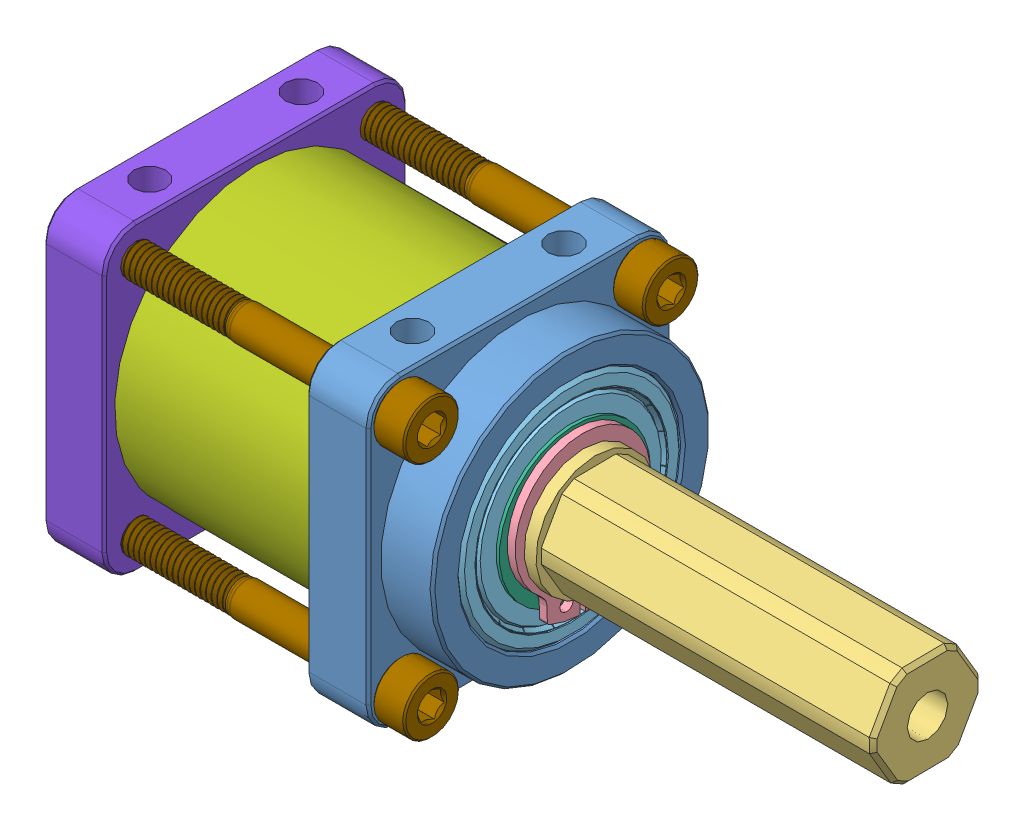
SolidWorks assembly Repeat Drive Magnum_V1.2, configuration Default. Lengths in mm.
Overall size (92.02 38.7 38.7).
14 component instances, 9 part files, 0 mates.
Components (placement in the parent):
- Repeat Drive Magnum_V1.2(2)^Repeat Drive Magnum_V1.2-1: Repeat Drive Magnum_V1.2(2)^Repeat Drive Magnum_V1.2 [Default] at origin size (92.02 38.7 38.7) (virtual)
  - 0500 Front V5^Repeat Drive Magnum_V1.2(2)_Repeat Drive Magnum_V1.2-1: 0500 Front V5^Repeat Drive Magnum_V1.2(2)_Repeat Drive Magnum_V1.2 [Default] at origin size (64.7 38.1 38.1) (virtual)
    - Faceplate 0500in v5^0500 Front V5_Repeat Drive Magnum_V1.2(2)_Repeat Drive Magnum_V1.2-1: Faceplate 0500in v5^0500 Front V5_Repeat Drive Magnum_V1.2(2)_Repeat Drive Magnum_V1.2 [Default] at origin (virtual)
    - 5972K155_Ball Bearing_5972K155^0500 Front V5_Repeat Drive Magnum_V1.2(2)_Repeat Drive Magnum_V1.2-1: 5972K155_Ball Bearing_5972K155^0500 Front V5_Repeat Drive Magnum_V1.2(2)_Repeat Drive Magnum_V1.2 [Default] at (1.5 0 0) x (0 0.98296 -0.183819) z (1 0 0) (virtual)
    - Shaft Mk2 0500 v5^0500 Front V5_Repeat Drive Magnum_V1.2(2)_Repeat Drive Magnum_V1.2-1: Shaft Mk2 0500 v5^0500 Front V5_Repeat Drive Magnum_V1.2(2)_Repeat Drive Magnum_V1.2 [Default] at (-5.7 0 0) x (0 0.01095 -0.99994) z (1 0 0) (virtual)
    - 98541A410_External Retaining Ring_98541A410^0500 Front V5_Repeat Drive Magnum_V1.2(2)_Repeat Drive Magnum_V1.2-1: 98541A410_External Retaining Ring_98541A410^0500 Front V5_Repeat Drive Magnum_V1.2(2)_Repeat Drive Magnum_V1.2 [Default] at (15.1875 0 0) x (0 0 1) z (-1 0 0) (virtual)
    - 5972K166_Ball Bearing_5972K166^0500 Front V5_Repeat Drive Magnum_V1.2(2)_Repeat Drive Magnum_V1.2-1: 5972K166_Ball Bearing_5972K166^0500 Front V5_Repeat Drive Magnum_V1.2(2)_Repeat Drive Magnum_V1.2 [Default] at (10.7875 0 0) x (0 0.013667 0.999907) z (-1 0 0) (virtual)
    - Shaft Washer Mk6^0500 Front V5_Repeat Drive Magnum_V1.2(2)_Repeat Drive Magnum_V1.2-1: Shaft Washer Mk6^0500 Front V5_Repeat Drive Magnum_V1.2(2)_Repeat Drive Magnum_V1.2 [Default] at (14.2875 0 0) x (0 0 -1) z (1 0 0) (virtual)
  - Ring Gear Mk2^Repeat Drive Magnum_V1.2(2)_Repeat Drive Magnum_V1.2-1: Ring Gear Mk2^Repeat Drive Magnum_V1.2(2)_Repeat Drive Magnum_V1.2 [Default] x (0 1 0) z (-1 0 0) (virtual)
  - Back Plate mk2^Repeat Drive Magnum_V1.2(2)_Repeat Drive Magnum_V1.2-1: Back Plate mk2^Repeat Drive Magnum_V1.2(2)_Repeat Drive Magnum_V1.2 [Default] at (-29.21 0 0) (virtual)
  - M4_91290A184^Repeat Drive Magnum_V1.2(2)_Repeat Drive Magnum_V1.2-1: M4_91290A184^Repeat Drive Magnum_V1.2(2)_Repeat Drive Magnum_V1.2 [Default] at (-10.2125 15.05 -15.05) x (0 -0.964256 0.264973) z (1 0 0) (virtual)
  - M4_91290A184^Repeat Drive Magnum_V1.2(2)_Repeat Drive Magnum_V1.2-2: M4_91290A184^Repeat Drive Magnum_V1.2(2)_Repeat Drive Magnum_V1.2 [Default] at (-10.2125 -15.05 -15.05) x (0 0.264973 0.964256) z (1 0 0) (virtual)
  - M4_91290A184^Repeat Drive Magnum_V1.2(2)_Repeat Drive Magnum_V1.2-3: M4_91290A184^Repeat Drive Magnum_V1.2(2)_Repeat Drive Magnum_V1.2 [Default] at (-10.2125 -15.05 15.05) x (0 0.964256 -0.264973) z (1 0 0) (virtual)
  - M4_91290A184^Repeat Drive Magnum_V1.2(2)_Repeat Drive Magnum_V1.2-4: M4_91290A184^Repeat Drive Magnum_V1.2(2)_Repeat Drive Magnum_V1.2 [Default] at (-10.2125 15.05 15.05) x (0 -0.264973 -0.964256) z (1 0 0) (virtual)
